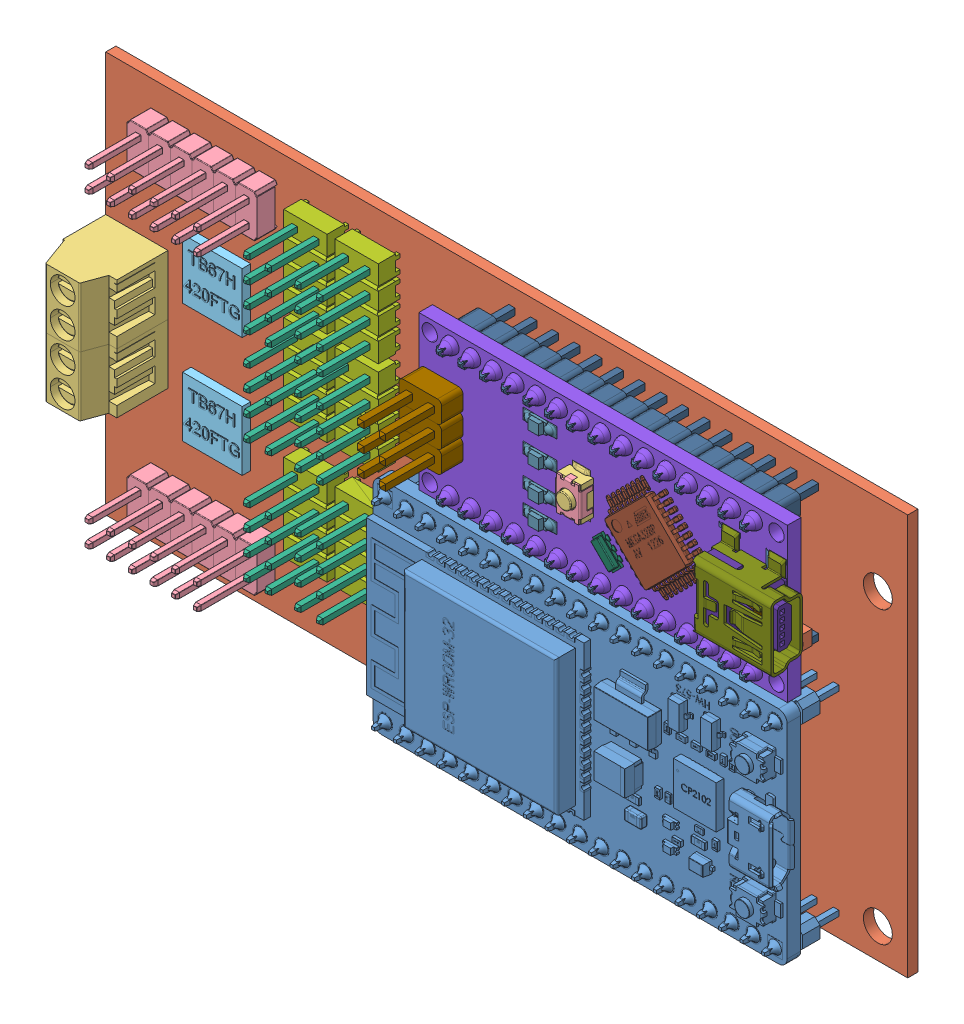
SolidWorks assembly Motor board, configuration Default. Lengths in mm.
Overall size (94 47 19.1).
66 component instances, 26 part files, 33 mates.
Components (placement in the parent):
- ESP32S Dev Board 0.9inch width ASSY-1: ESP32S Dev Board 0.9inch width ASSY [Default] at (-31.257 13.954 6.74) x (0 1 0) z (1 0 0) size (25.91 13.14 49.31)
- Motor PCB-1: Motor PCB [Default] at (-47 23.5 0) x (-1 0 0) z (0 0 1) size (94 47 1.2)
- 2pos-3.5mm-term-blk.stp-1: 2pos-3.5mm-term-blk.stp [Default] at (-94 27 3.6) x (0 -1 0) z (-1 0 0) size (7 12 7.3)
- 2x6-100mil-male-header.step-1: 2x6-100mil-male-header.step [Default] at (-87.73 41.5 2.45) x (-1 0 0) z (0 1 0) size (15.24 11.55 5)
- 2x6-100mil-male-header.step-2: 2x6-100mil-male-header.step [Default] at (-87.73 5.5 2.45) x (-1 0 0) z (0 1 0) size (15.24 11.55 5)
- 2pos-3.5mm-term-blk.stp-2: 2pos-3.5mm-term-blk.stp [Default] at (-94 20 3.6) x (0 -1 0) z (-1 0 0) size (7 12 7.3)
- TB67H420FTG-1: TB67H420FTG [Default] at (-80.5 30.5 1.2) size (7 7 1.1)
- TB67H420FTG-2: TB67H420FTG [Default] at (-80.5 16.5 1.2) size (7 7 1.1)
- 2x4 100mil male header-1: 2x4 100mil male header [Default] at (-68.054 38.92 1.2) x (0 1 0) z (1 0 0) size (10.16 10.92 5.08)
  - TSW_104_07_T_D_3-1: TSW_104_07_T_D_3 [Default] at (0 -2.54 0) size (8.51 10.92 3.43)
  - TSW_104_07_T_D_5-1: TSW_104_07_T_D_5 [Default] at origin size (10.16 2.54 5.08)
- 2x4 100mil male header-3: 2x4 100mil male header [Default] at (-62.054 38.92 1.2) x (0 1 0) z (1 0 0) size (10.16 10.92 5.08)
  - TSW_104_07_T_D_3-1: TSW_104_07_T_D_3 [Default] at (0 -2.54 0) size (8.51 10.92 3.43)
  - TSW_104_07_T_D_5-1: TSW_104_07_T_D_5 [Default] at origin size (10.16 2.54 5.08)
- Arduino Nano v3-1: Arduino Nano v3 [Default] at (-46.38 29.38 6.7) x (1 0 0) z (0 -1 0) size (45 18.6 18)
  - nano-board-1: nano-board [Default] at origin size (43.2 4.6 18)
  - 2pin_header__02-1: 2pin_header__02 [Default] at (-1.143 1.6 -7.62) size (5 11.75 2.54)
  - 2pin_header__02-2: 2pin_header__02 [Default] at (-1.143 1.6 -5.08) size (5 11.75 2.54)
  - 2pin_header__02-3: 2pin_header__02 [Default] at (-1.143 1.6 -10.16) size (5 11.75 2.54)
  - 15pin_header__-1: 15pin_header__ [Default] x (0 0 1) z (1 0 0) size (2.54 11.75 38.1)
  - 15pin_header__-2: 15pin_header__ [Default] at (0 0 -15.24) x (0 0 1) z (1 0 0) size (2.54 11.75 38.1)
  - atmega328-1: atmega328 [Default] at (23.85 1.75 -7.62) x (-0.707107 0 0.707107) z (-0.707107 0 -0.707107) size (10 1.1 10)
  - ftdi FT232rl-1: ftdi FT232rl [Default] at (29.05 0 -7.67) x (0 0 -1) z (-1 0 0) size (9.25 1.9 10.2)
  - smt_resistor222-10: smt_resistor222 [Default] at (21.86 0 -5.8) x (0 0 -1) z (-1 0 0) size (1.7 0.6 3.8)
  - smt_resistor222-6: smt_resistor222 [Default] at (21.86 0 -9) x (0 0 -1) z (-1 0 0) size (1.7 0.6 3.8)
  - smt_resistor222-8: smt_resistor222 [Default] at (36.75 0 -7.6) x (0 0 -1) z (-1 0 0) size (1.7 0.6 3.8)
  - smt_resistor222-9: smt_resistor222 [Default] at (36.75 0 -12) x (0 0 -1) z (-1 0 0) size (1.7 0.6 3.8)
  - smt_resistor222-7: smt_resistor222 [Default] at (8.2 0 -2.6) x (0 0 -1) z (-1 0 0) size (1.7 0.6 3.8)
  - led-1: led [Default] at (10.4 1.6 -2.8) size (4 0.86 1.35)
  - led-2: led [Default] at (10.4 1.6 -5.55) size (4 0.86 1.35)
  - led-3: led [Default] at (10.4 1.6 -12.5) size (4 0.86 1.35)
  - led-4: led [Default] at (10.4 1.6 -9.05) size (4 0.86 1.35)
  - 16mhz crystal - measured-1: 16mhz crystal - measured [Default] at (18.5113 1.6 -3.5541) x (0.707107 0 0.707107) z (-0.707107 0 0.707107) size (3.4 0.8 2)
  - MINIUSB - MEASURED-1: MINIUSB - MEASURED [Default] at (38.98 1.65 -7.62) x (0 0 1) z (-1 0 0) size (10.9 4.8 10.41)
    - MINIUSBSHELL-1: MINIUSBSHELL [Default] at origin size (10.9 3.75 9.4)
    - MINIUSBCORE-1: MINIUSBCORE [Default] at (0 0 6.7) x (-1 0 0) z (0 0 -1) size (7.7 4.5 8.2)
    - MINI USB CONTACT-1: MINI USB CONTACT [Default] at (-1.6 0 5.7) x (-1 0 0) z (0 0 -1) size (0.51 2.56 9.41)
    - MINI USB CONTACT-2: MINI USB CONTACT [Default] at (-0.8 0 5.7) x (-1 0 0) z (0 0 -1) size (0.51 2.56 9.41)
    - MINI USB CONTACT-3: MINI USB CONTACT [Default] at (0 0 5.7) x (-1 0 0) z (0 0 -1) size (0.51 2.56 9.41)
    - MINI USB CONTACT-4: MINI USB CONTACT [Default] at (0.8 0 5.7) x (-1 0 0) z (0 0 -1) size (0.51 2.56 9.41)
    - MINI USB CONTACT-5: MINI USB CONTACT [Default] at (1.6 0 5.7) x (-1 0 0) z (0 0 -1) size (0.51 2.56 9.41)
    - MINI USB SOLDER-1: MINI USB SOLDER [Default] at (0 -0.05 -0.4) x (-1 0 0) z (0 0 -1) size (10.9 0.01 8)
  - cap106C-1: cap106C [Default] at (37.2 0 -3.3) x (0 0 1) z (1 0 0) size (1.7 1.81 4)
  - cap106C-2: cap106C [Default] at (7.9 0 -5.6) x (0 0 -1) z (-1 0 0) size (1.7 1.81 4)
  - reset button-1: reset button [Default] at (15.25 1.6 -8.05) x (0 0 -1) z (1 0 0) size (5.2 2.15 3)
    - reset core-1: reset core [Default] at origin size (5.2 2.15 2.8)
    - reset shell-1: reset shell [Default] at (0 1.65 0) x (0 0 1) z (-1 0 0) size (3 1.65 4)
  - nano - reg-1: nano - reg [Default] at (6.1 0 -10.16) x (0 0 -1) z (-1 0 0) size (6.5 1.69 8.3)
  - NANO DIODE-1: NANO DIODE [Default] at (11.43 0 -4.2) x (0 0 1) z (1 0 0) size (4.92 1.36 1.7)
  - 189 RESISTOR PACK-1: 189 RESISTOR PACK [Default] at (15.75 0 -10.85) x (0 0 1) z (1 0 0) size (3.2 0.46 3)
  - 102 RESISTOR PACK-1: 102 RESISTOR PACK [Default] at (15.75 0 -5.2) x (0 0 1) z (1 0 0) size (3.2 0.46 3)
- 2x4 100mil male header-6: 2x4 100mil male header [Default] at (-68.054 27.92 1.2) x (0 1 0) z (1 0 0) size (10.16 10.92 5.08)
  - TSW_104_07_T_D_3-1: TSW_104_07_T_D_3 [Default] at (0 -2.54 0) size (8.51 10.92 3.43)
  - TSW_104_07_T_D_5-1: TSW_104_07_T_D_5 [Default] at origin size (10.16 2.54 5.08)
- 2x4 100mil male header-7: 2x4 100mil male header [Default] at (-62.054 27.92 1.2) x (0 1 0) z (1 0 0) size (10.16 10.92 5.08)
  - TSW_104_07_T_D_3-1: TSW_104_07_T_D_3 [Default] at (0 -2.54 0) size (8.51 10.92 3.43)
  - TSW_104_07_T_D_5-1: TSW_104_07_T_D_5 [Default] at origin size (10.16 2.54 5.08)
- 2x4 100mil male header-10: 2x4 100mil male header [Default] at (-68.054 13.76 1.2) x (0 1 0) z (1 0 0) size (10.16 10.92 5.08)
  - TSW_104_07_T_D_3-1: TSW_104_07_T_D_3 [Default] at (0 -2.54 0) size (8.51 10.92 3.43)
  - TSW_104_07_T_D_5-1: TSW_104_07_T_D_5 [Default] at origin size (10.16 2.54 5.08)
- 2x4 100mil male header-11: 2x4 100mil male header [Default] at (-62.054 13.76 1.2) x (0 1 0) z (1 0 0) size (10.16 10.92 5.08)
  - TSW_104_07_T_D_3-1: TSW_104_07_T_D_3 [Default] at (0 -2.54 0) size (8.51 10.92 3.43)
  - TSW_104_07_T_D_5-1: TSW_104_07_T_D_5 [Default] at origin size (10.16 2.54 5.08)
- 2x4 100mil male header-12: 2x4 100mil male header [Default] at (-62.054 13.76 1.2) x (0 1 0) z (1 0 0) size (10.16 10.92 5.08)
  - TSW_104_07_T_D_3-1: TSW_104_07_T_D_3 [Default] at (0 -2.54 0) size (8.51 10.92 3.43)
  - TSW_104_07_T_D_5-1: TSW_104_07_T_D_5 [Default] at origin size (10.16 2.54 5.08)
Mates (geometry in assembly coordinates):
- Distance13: distance = 3 mm anti-aligned: plane of ESP32S Dev Board 0.9inch width ASSY-1 through (-56.4432 26.7247 4.2) normal (0 0 -1); plane of Motor PCB-1 through (-47 23.5 1.2) normal (0 0 1)
- Distance18: distance = 7 mm aligned: plane of ESP32S Dev Board 0.9inch width ASSY-1 through (-7 1 8.34) normal (1 0 0); plane of Motor PCB-1 through (0 0 1.2) normal (1 0 0)
- Coincident5: coincident anti-aligned: plane of Motor PCB-1 through (-47 23.5 1.2) normal (0 0 1); plane of 2pos-3.5mm-term-blk.stp-1 through (-94 30.5 1.2) normal (0 0 -1)
- Coincident6: coincident aligned: plane of Motor PCB-1 through (-94 0 1.2) normal (-1 0 0); plane of 2pos-3.5mm-term-blk.stp-1 through (-94 30.5 6.2) normal (-1 0 0)
- Distance25: distance = 16.5 mm aligned: plane of Motor PCB-1 through (0 47 1.2) normal (0 1 0); plane of 2pos-3.5mm-term-blk.stp-1 through (-94 30.5 3.6) normal (0 1 0)
- Coincident8: coincident anti-aligned: plane of Motor PCB-1 through (-47 23.5 1.2) normal (0 0 1); plane of 2x6-100mil-male-header.step-1 through (-86.1089 39.06 1.2) normal (0 0 -1)
- Distance14: distance = 1 mm aligned: plane of Motor PCB-1 through (0 0 1.2) normal (0 -1 0); plane of ESP32S Dev Board 0.9inch width ASSY-1 through (-55.514 1 8.34) normal (0 -1 0)
- Coincident21: coincident anti-aligned: plane of Motor PCB-1 through (-47 23.5 1.2) normal (0 0 1); plane of 2x6-100mil-male-header.step-2 through (-75.9489 3.06 1.2) normal (0 0 -1)
- Coincident29: coincident anti-aligned: plane of Motor PCB-1 through (-47 23.5 1.2) normal (0 0 1); plane of 2pos-3.5mm-term-blk.stp-2 through (-94 23.5 1.2) normal (0 0 -1)
- Coincident30: coincident aligned: plane of 2pos-3.5mm-term-blk.stp-1 through (-94 30.5 6.2) normal (-1 0 0); plane of 2pos-3.5mm-term-blk.stp-2 through (-94 23.5 6.2) normal (-1 0 0)
- Coincident32: coincident anti-aligned: plane of 2pos-3.5mm-term-blk.stp-1 through (-94 23.5 3.6) normal (0 -1 0); plane of 2pos-3.5mm-term-blk.stp-2 through (-94 23.5 3.6) normal (0 1 0)
- Coincident35: coincident anti-aligned: plane of Motor PCB-1 through (-47 23.5 1.2) normal (0 0 1); plane of TB67H420FTG-1 through (-80.5 30.5 1.2) normal (0 0 -1)
- Distance8: distance = 5 mm: plane of TB67H420FTG-1 through (-84 34 2.2) normal (0 1 0); plane of 2x6-100mil-male-header.step-1 through (-81.7311 39 3.7) normal (0 -1 0)
- Distance9: distance = 5 mm aligned: plane of TB67H420FTG-1 through (-84 34 2.2) normal (-1 0 0); plane of 2x6-100mil-male-header.step-1 through (-89 39.375 3.7) normal (-1 0 0)
- Coincident40: coincident anti-aligned: plane of Motor PCB-1 through (-47 23.5 1.2) normal (0 0 1); plane of TB67H420FTG-2 through (-80.5 16.5 1.2) normal (0 0 -1)
- Coincident43: coincident anti-aligned: plane of Motor PCB-1 through (-47 23.5 1.2) normal (0 0 1); plane of 2x4 100mil male header-1/TSW_104_07_T_D_5-1 through (-68.054 38.92 1.2) normal (0 0 -1)
- Distance19: distance = 3 mm anti-aligned: plane of Motor PCB-1 through (-47 23.5 1.2) normal (0 0 1); plane of Arduino Nano v3-1/15pin_header__-1 through (-45.61 28.61 4.2) normal (0 0 -1)
- Coincident56: coincident anti-aligned: plane of Motor PCB-1 through (0 0 1.2) normal (0 -1 0)
- Coincident57: coincident aligned: plane of Motor PCB-1 through (0 0 1.2) normal (1 0 0)
- Coincident58: coincident anti-aligned: plane of Motor PCB-1 through (-47 23.5 0) normal (0 0 -1)
- Distance21: distance = 1 mm aligned: plane of Motor PCB-1 through (0 47 1.2) normal (0 1 0); plane of Arduino Nano v3-1/nano-board-1 through (-50.2 46 8.3) normal (0 1 0)
- Distance15: distance = 7 mm anti-aligned: plane of TB67H420FTG-2 through (-84 20 2.2) normal (0 1 0); plane of TB67H420FTG-1 through (-84 27 2.2) normal (0 -1 0)
- Coincident62: coincident aligned: plane of TB67H420FTG-1 through (-84 34 2.2) normal (-1 0 0); plane of TB67H420FTG-2 through (-84 20 2.2) normal (-1 0 0)
- Distance16: distance = 5 mm anti-aligned: plane of TB67H420FTG-2 through (-84 13 2.2) normal (0 -1 0); plane of 2x6-100mil-male-header.step-2 through (-86.8111 8 3.7) normal (0 1 0)
- Coincident64: coincident aligned: plane of 2x6-100mil-male-header.step-1 through (-89 39.375 3.7) normal (-1 0 0); plane of 2x6-100mil-male-header.step-2 through (-89 3.375 3.7) normal (-1 0 0)
- Coincident67: coincident aligned: plane of ESP32S Dev Board 0.9inch width ASSY-1 through (-7 1 8.34) normal (1 0 0); plane of Arduino Nano v3-1/nano-board-1 through (-7 46 8.3) normal (1 0 0)
- Distance23: distance = 3 mm aligned: plane of Motor PCB-1 through (0 47 1.2) normal (0 1 0); plane of 2x4 100mil male header-1/TSW_104_07_T_D_5-1 through (-65.514 44 3.74) normal (0 1 0)
- Distance24: distance = 10 mm anti-aligned: plane of 2x4 100mil male header-1/TSW_104_07_T_D_5-1 through (-65.514 33.84 3.74) normal (1 0 0); plane of ESP32S Dev Board 0.9inch width ASSY-1 through (-55.514 1 8.34) normal (-1 0 0)
- Distance28: distance = 3 mm aligned: plane of Motor PCB-1 through (0 0 1.2) normal (0 -1 0); plane of 2x6-100mil-male-header.step-2 through (-79.1911 3 3.7) normal (0 -1 0)
- Distance27: distance = 5 mm aligned: plane of Motor PCB-1 through (-94 0 1.2) normal (-1 0 0); plane of 2x6-100mil-male-header.step-2 through (-89 3.375 3.7) normal (-1 0 0)
- Coincident69: coincident aligned: plane of 2x4 100mil male header-6/TSW_104_07_T_D_5-1 through (-70.594 33 3.74) normal (-1 0 0); plane of 2x4 100mil male header-10/TSW_104_07_T_D_5-1 through (-70.594 18.84 3.74) normal (-1 0 0)
- Distance31: distance = 4 mm anti-aligned: plane of 2x4 100mil male header-6/TSW_104_07_T_D_5-1 through (-70.594 22.84 3.74) normal (0 -1 0); plane of 2x4 100mil male header-10/TSW_104_07_T_D_5-1 through (-65.514 18.84 3.74) normal (0 1 0)
- Coincident71: coincident anti-aligned: plane of Motor PCB-1 through (-47 23.5 1.2) normal (0 0 1); plane of 2x4 100mil male header-10/TSW_104_07_T_D_5-1 through (-68.054 13.76 1.2) normal (0 0 -1)
